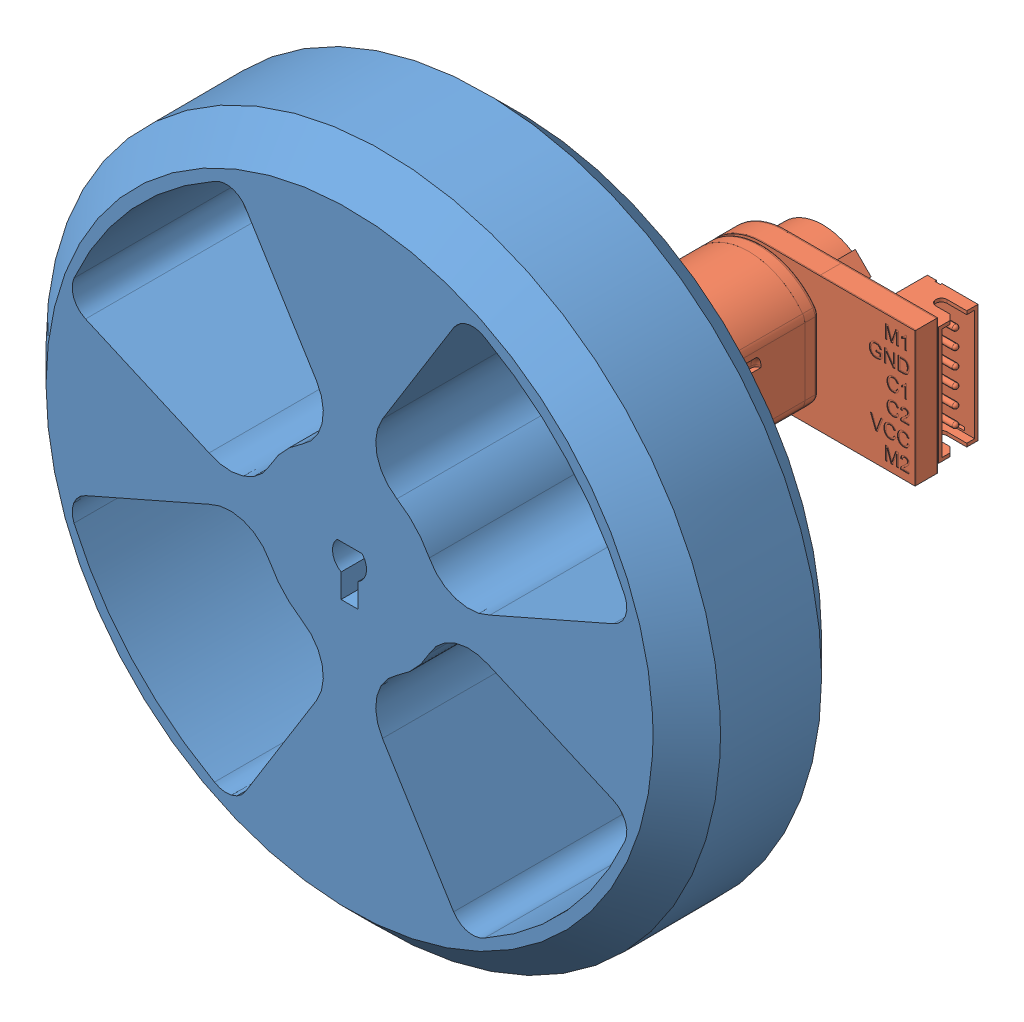
SolidWorks assembly Assem1, configuration Default. Lengths in mm.
Overall size (60 60 42.4).
2 component instances, 2 part files, 0 mates.
Components (placement in the parent):
- Part1-1: Part1 [Default] at (6.6149 4.7022 60) size (60 60 15)
- N20 Mini Micro Metall Gear Motor DC 3-6-12V v1.step-1: N20 Mini Micro Metall Gear Motor DC 3-6-12V v1.step [Default] at (6.6222 4.7046 53.3979) x (0 0 1) z (1 0 0) size (39.8 12.15 18.58)
